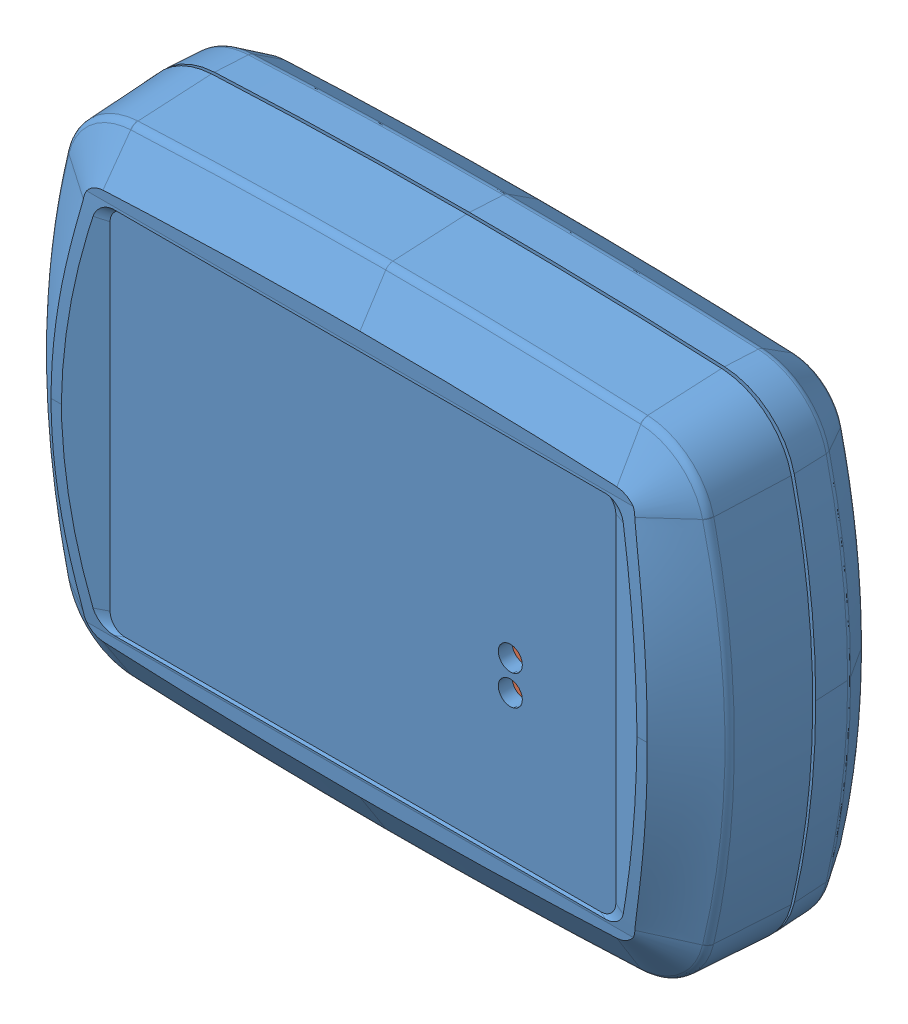
SolidWorks assembly СБ Peggy Receiver, configuration Default. Lengths in mm. (continued)
Components (placement in the parent): (continued)
- Печатная плата Peggy Receiver-1: Печатная плата Peggy Receiver [Default] at (11919.9713 53.7301 2.2215) x (0.000006 1 0) z (0 0 1) size (75.31 78.06 11.44) (continued)
  - Печатная плата Peggy Receiver(2)^Печатная плата Peggy Receiver-2: Печатная плата Peggy Receiver(2)^Печатная плата Peggy Receiver [Default] at origin size (75.31 78.06 11.44) (virtual) (continued)
    - DD1^Печатная плата Peggy Receiver(2)_Печатная плата Peggy Receiver-2: DD1^Печатная плата Peggy Receiver(2)_Печатная плата Peggy Receiver [Default] at origin size (16 15.9 2.23) (virtual) (continued)
      - User Library-RFM96W^DD1_Печатная плата Peggy Receiver(2)_Печатная плата Peggy Receiver-1: User Library-RFM96W^DD1_Печатная плата Peggy Receiver(2)_Печатная плата Peggy Receiver [Default] at (17.298 57.975 1.15) x (1 0 0) z (0 0 1) size (16 15.9 2.23) (virtual) (continued)
        - Designator9^User Library-RFM96W_DD1_Печатная плата Peggy Receiver(2)_Печатная плата Peggy Receiver-1: Designator9^User Library-RFM96W_DD1_Печатная плата Peggy Receiver(2)_Печатная плата Peggy Receiver [Default] at origin size (0.5 1 0.5) (virtual)
          - Cap0402^Designator9_User Library-RFM96W_DD1_Печатная плата Peggy Receiver(2)_Печатная плата Peggy Receiver-1: Cap0402^Designator9_User Library-RFM96W_DD1_Печатная плата Peggy Receiver(2)_Печатная плата Peggy Receiver [Default] at (2.8 5.98 0) x (0 -1 0) z (-1 0 0) size (1 0.5 0.5) (virtual)
        - Designator10^User Library-RFM96W_DD1_Печатная плата Peggy Receiver(2)_Печатная плата Peggy Receiver-1: Designator10^User Library-RFM96W_DD1_Печатная плата Peggy Receiver(2)_Печатная плата Peggy Receiver [Default] at origin size (0.5 1 0.5) (virtual)
          - Cap0402^Designator10_User Library-RFM96W_DD1_Печатная плата Peggy Receiver(2)_Печатная плата Peggy Receiver-1: Cap0402^Designator10_User Library-RFM96W_DD1_Печатная плата Peggy Receiver(2)_Печатная плата Peggy Receiver [Default] at (4.953 6.858 0) x (0 -1 0) z (-1 0 0) size (1 0.5 0.5) (virtual)
        - Designator11^User Library-RFM96W_DD1_Печатная плата Peggy Receiver(2)_Печатная плата Peggy Receiver-1: Designator11^User Library-RFM96W_DD1_Печатная плата Peggy Receiver(2)_Печатная плата Peggy Receiver [Default] at origin size (0.5 1 0.5) (virtual)
          - Cap0402^Designator11_User Library-RFM96W_DD1_Печатная плата Peggy Receiver(2)_Печатная плата Peggy Receiver-1: Cap0402^Designator11_User Library-RFM96W_DD1_Печатная плата Peggy Receiver(2)_Печатная плата Peggy Receiver [Default] at (6.35 11.557 0) x (0 1 0) z (1 0 0) size (1 0.5 0.5) (virtual)
        - Designator12^User Library-RFM96W_DD1_Печатная плата Peggy Receiver(2)_Печатная плата Peggy Receiver-1: Designator12^User Library-RFM96W_DD1_Печатная плата Peggy Receiver(2)_Печатная плата Peggy Receiver [Default] at origin size (1 0.5 0.5) (virtual)
          - Cap0402^Designator12_User Library-RFM96W_DD1_Печатная плата Peggy Receiver(2)_Печатная плата Peggy Receiver-1: Cap0402^Designator12_User Library-RFM96W_DD1_Печатная плата Peggy Receiver(2)_Печатная плата Peggy Receiver [Default] at (5.461 8.128 0) x (1 0 0) z (0 -1 0) size (1 0.5 0.5) (virtual)
        - Designator13^User Library-RFM96W_DD1_Печатная плата Peggy Receiver(2)_Печатная плата Peggy Receiver-1: Designator13^User Library-RFM96W_DD1_Печатная плата Peggy Receiver(2)_Печатная плата Peggy Receiver [Default] at origin size (0.5 1 0.5) (virtual)
          - Cap0402^Designator13_User Library-RFM96W_DD1_Печатная плата Peggy Receiver(2)_Печатная плата Peggy Receiver-1: Cap0402^Designator13_User Library-RFM96W_DD1_Печатная плата Peggy Receiver(2)_Печатная плата Peggy Receiver [Default] at (3.937 6.858 0) x (0 1 0) z (1 0 0) size (1 0.5 0.5) (virtual)
        - Designator15^User Library-RFM96W_DD1_Печатная плата Peggy Receiver(2)_Печатная плата Peggy Receiver-1: Designator15^User Library-RFM96W_DD1_Печатная плата Peggy Receiver(2)_Печатная плата Peggy Receiver [Default] at origin size (0.52 1.02 0.37) (virtual)
          - SW3dPS-inductor_0402_white^Designator15_User Library-RFM96W_DD1_Печатная плата Peggy Receiver(2)_Печатная плата Peggy Receiver-1: SW3dPS-inductor_0402_white^Designator15_User Library-RFM96W_DD1_Печатная плата Peggy Receiver(2)_Печатная плата Peggy Receiver [Default] at (13.208 12.446 0) x (1 0 0) z (0 -1 0) size (0.52 0.37 1.02) (virtual)
        - Designator17^User Library-RFM96W_DD1_Печатная плата Peggy Receiver(2)_Печатная плата Peggy Receiver-1: Designator17^User Library-RFM96W_DD1_Печатная плата Peggy Receiver(2)_Печатная плата Peggy Receiver [Default] at origin size (1.02 0.52 0.37) (virtual)
          - SW3dPS-inductor_0402_white^Designator17_User Library-RFM96W_DD1_Печатная плата Peggy Receiver(2)_Печатная плата Peggy Receiver-1: SW3dPS-inductor_0402_white^Designator17_User Library-RFM96W_DD1_Печатная плата Peggy Receiver(2)_Печатная плата Peggy Receiver [Default] at (8.636 8.89 0) x (0 1 0) z (1 0 0) size (0.52 0.37 1.02) (virtual)
        - Designator18^User Library-RFM96W_DD1_Печатная плата Peggy Receiver(2)_Печатная плата Peggy Receiver-1: Designator18^User Library-RFM96W_DD1_Печатная плата Peggy Receiver(2)_Печатная плата Peggy Receiver [Default] at origin size (1.02 0.52 0.37) (virtual)
          - SW3dPS-inductor_0402_white^Designator18_User Library-RFM96W_DD1_Печатная плата Peggy Receiver(2)_Печатная плата Peggy Receiver-1: SW3dPS-inductor_0402_white^Designator18_User Library-RFM96W_DD1_Печатная плата Peggy Receiver(2)_Печатная плата Peggy Receiver [Default] at (9.398 10.414 0) x (0 1 0) z (1 0 0) size (0.52 0.37 1.02) (virtual)
        - Designator19^User Library-RFM96W_DD1_Печатная плата Peggy Receiver(2)_Печатная плата Peggy Receiver-1: Designator19^User Library-RFM96W_DD1_Печатная плата Peggy Receiver(2)_Печатная плата Peggy Receiver [Default] at origin size (1.02 0.52 0.37) (virtual)
          - SW3dPS-inductor_0402_white^Designator19_User Library-RFM96W_DD1_Печатная плата Peggy Receiver(2)_Печатная плата Peggy Receiver-1: SW3dPS-inductor_0402_white^Designator19_User Library-RFM96W_DD1_Печатная плата Peggy Receiver(2)_Печатная плата Peggy Receiver [Default] at (8.636 12.319 0) x (0 1 0) z (1 0 0) size (0.52 0.37 1.02) (virtual)
        - Designator20^User Library-RFM96W_DD1_Печатная плата Peggy Receiver(2)_Печатная плата Peggy Receiver-1: Designator20^User Library-RFM96W_DD1_Печатная плата Peggy Receiver(2)_Печатная плата Peggy Receiver [Default] at origin size (1.02 0.52 0.37) (virtual)
          - SW3dPS-inductor_0402_white^Designator20_User Library-RFM96W_DD1_Печатная плата Peggy Receiver(2)_Печатная плата Peggy Receiver-1: SW3dPS-inductor_0402_white^Designator20_User Library-RFM96W_DD1_Печатная плата Peggy Receiver(2)_Печатная плата Peggy Receiver [Default] at (10.668 12.319 0) x (0 1 0) z (1 0 0) size (0.52 0.37 1.02) (virtual)
        - Designator21^User Library-RFM96W_DD1_Печатная плата Peggy Receiver(2)_Печатная плата Peggy Receiver-1: Designator21^User Library-RFM96W_DD1_Печатная плата Peggy Receiver(2)_Печатная плата Peggy Receiver [Default] at origin size (1 0.5 0.5) (virtual)
          - Cap0402^Designator21_User Library-RFM96W_DD1_Печатная плата Peggy Receiver(2)_Печатная плата Peggy Receiver-1: Cap0402^Designator21_User Library-RFM96W_DD1_Печатная плата Peggy Receiver(2)_Печатная плата Peggy Receiver [Default] at (10.668 10.414 0) x (-1 0 0) z (0 1 0) size (1 0.5 0.5) (virtual)
        - Designator22^User Library-RFM96W_DD1_Печатная плата Peggy Receiver(2)_Печатная плата Peggy Receiver-1: Designator22^User Library-RFM96W_DD1_Печатная плата Peggy Receiver(2)_Печатная плата Peggy Receiver [Default] at origin size (0.5 1 0.5) (virtual)
          - Cap0402^Designator22_User Library-RFM96W_DD1_Печатная плата Peggy Receiver(2)_Печатная плата Peggy Receiver-1: Cap0402^Designator22_User Library-RFM96W_DD1_Печатная плата Peggy Receiver(2)_Печатная плата Peggy Receiver [Default] at (8.255 10.922 0) x (0 1 0) z (1 0 0) size (1 0.5 0.5) (virtual)
        - Designator23^User Library-RFM96W_DD1_Печатная плата Peggy Receiver(2)_Печатная плата Peggy Receiver-1: Designator23^User Library-RFM96W_DD1_Печатная плата Peggy Receiver(2)_Печатная плата Peggy Receiver [Default] at origin size (1 0.5 0.5) (virtual)
          - Cap0402^Designator23_User Library-RFM96W_DD1_Печатная плата Peggy Receiver(2)_Печатная плата Peggy Receiver-1: Cap0402^Designator23_User Library-RFM96W_DD1_Печатная плата Peggy Receiver(2)_Печатная плата Peggy Receiver [Default] at (6.858 14.859 0) x (-1 0 0) z (0 1 0) size (1 0.5 0.5) (virtual)
        - Designator24^User Library-RFM96W_DD1_Печатная плата Peggy Receiver(2)_Печатная плата Peggy Receiver-1: Designator24^User Library-RFM96W_DD1_Печатная плата Peggy Receiver(2)_Печатная плата Peggy Receiver [Default] at origin size (1 0.5 0.5) (virtual)
          - Cap0402^Designator24_User Library-RFM96W_DD1_Печатная плата Peggy Receiver(2)_Печатная плата Peggy Receiver-1: Cap0402^Designator24_User Library-RFM96W_DD1_Печатная плата Peggy Receiver(2)_Печатная плата Peggy Receiver [Default] at (12.827 13.843 0) x (-1 0 0) z (0 1 0) size (1 0.5 0.5) (virtual)
        - Designator25^User Library-RFM96W_DD1_Печатная плата Peggy Receiver(2)_Печатная плата Peggy Receiver-1: Designator25^User Library-RFM96W_DD1_Печатная плата Peggy Receiver(2)_Печатная плата Peggy Receiver [Default] at origin size (0.5 1 0.5) (virtual)
          - Cap0402^Designator25_User Library-RFM96W_DD1_Печатная плата Peggy Receiver(2)_Печатная плата Peggy Receiver-1: Cap0402^Designator25_User Library-RFM96W_DD1_Печатная плата Peggy Receiver(2)_Печатная плата Peggy Receiver [Default] at (7.366 11.938 0) x (0 -1 0) z (-1 0 0) size (1 0.5 0.5) (virtual)
        - Designator26^User Library-RFM96W_DD1_Печатная плата Peggy Receiver(2)_Печатная плата Peggy Receiver-1: Designator26^User Library-RFM96W_DD1_Печатная плата Peggy Receiver(2)_Печатная плата Peggy Receiver [Default] at origin size (0.5 1 0.5) (virtual)
          - Cap0402^Designator26_User Library-RFM96W_DD1_Печатная плата Peggy Receiver(2)_Печатная плата Peggy Receiver-1: Cap0402^Designator26_User Library-RFM96W_DD1_Печатная плата Peggy Receiver(2)_Печатная плата Peggy Receiver [Default] at (12.319 12.446 0) x (0 -1 0) z (-1 0 0) size (1 0.5 0.5) (virtual)
        - Designator27^User Library-RFM96W_DD1_Печатная плата Peggy Receiver(2)_Печатная плата Peggy Receiver-1: Designator27^User Library-RFM96W_DD1_Печатная плата Peggy Receiver(2)_Печатная плата Peggy Receiver [Default] at origin size (1 0.5 0.5) (virtual)
          - Cap0402^Designator27_User Library-RFM96W_DD1_Печатная плата Peggy Receiver(2)_Печатная плата Peggy Receiver-1: Cap0402^Designator27_User Library-RFM96W_DD1_Печатная плата Peggy Receiver(2)_Печатная плата Peggy Receiver [Default] at (12.827 14.986 0) x (-1 0 0) z (0 1 0) size (1 0.5 0.5) (virtual)
        - Designator28^User Library-RFM96W_DD1_Печатная плата Peggy Receiver(2)_Печатная плата Peggy Receiver-1: Designator28^User Library-RFM96W_DD1_Печатная плата Peggy Receiver(2)_Печатная плата Peggy Receiver [Default] at origin size (0.5 1 0.5) (virtual)
          - Cap0402^Designator28_User Library-RFM96W_DD1_Печатная плата Peggy Receiver(2)_Печатная плата Peggy Receiver-1: Cap0402^Designator28_User Library-RFM96W_DD1_Печатная плата Peggy Receiver(2)_Печатная плата Peggy Receiver [Default] at (9.652 11.684 0) x (0 -1 0) z (-1 0 0) size (1 0.5 0.5) (virtual)
        - Designator29^User Library-RFM96W_DD1_Печатная плата Peggy Receiver(2)_Печатная плата Peggy Receiver-1: Designator29^User Library-RFM96W_DD1_Печатная плата Peggy Receiver(2)_Печатная плата Peggy Receiver [Default] at origin size (0.5 1 0.5) (virtual)
          - Cap0402^Designator29_User Library-RFM96W_DD1_Печатная плата Peggy Receiver(2)_Печатная плата Peggy Receiver-1: Cap0402^Designator29_User Library-RFM96W_DD1_Печатная плата Peggy Receiver(2)_Печатная плата Peggy Receiver [Default] at (13.208 9.779 0) x (0 -1 0) z (-1 0 0) size (1 0.5 0.5) (virtual)
        - Designator27_2^User Library-RFM96W_DD1_Печатная плата Peggy Receiver(2)_Печатная плата Peggy Receiver-1: Designator27_2^User Library-RFM96W_DD1_Печатная плата Peggy Receiver(2)_Печатная плата Peggy Receiver [Default] at origin size (2.43 2.79 1.09) (virtual)
          - SW3dPS-SOT-23-6^Designator27_2_User Library-RFM96W_DD1_Печатная плата Peggy Receiver(2)_Печатная плата Peggy Receiver-1: SW3dPS-SOT-23-6^Designator27_2_User Library-RFM96W_DD1_Печатная плата Peggy Receiver(2)_Печатная плата Peggy Receiver [Default] at (9.0742 15.0495 0) x (0 -1 0) z (0 0 1) size (2.79 2.43 1.09) (virtual)
        - Designator2^User Library-RFM96W_DD1_Печатная плата Peggy Receiver(2)_Печатная плата Peggy Receiver-1: Designator2^User Library-RFM96W_DD1_Печатная плата Peggy Receiver(2)_Печатная плата Peggy Receiver [Default] at origin size (5.04 5.04 0.9) (virtual)
          - QFN28^Designator2_User Library-RFM96W_DD1_Печатная плата Peggy Receiver(2)_Печатная плата Peggy Receiver-1: QFN28^Designator2_User Library-RFM96W_DD1_Печатная плата Peggy Receiver(2)_Печатная плата Peggy Receiver [Default] at (9.97 5.42 0) x (0 -1 0) z (-1 0 0) size (5.04 0.9 5.04) (virtual)
        - Designator5^User Library-RFM96W_DD1_Печатная плата Peggy Receiver(2)_Печатная плата Peggy Receiver-1: Designator5^User Library-RFM96W_DD1_Печатная плата Peggy Receiver(2)_Печатная плата Peggy Receiver [Default] at origin size (0.5 1 0.5) (virtual)
          - Cap0402^Designator5_User Library-RFM96W_DD1_Печатная плата Peggy Receiver(2)_Печатная плата Peggy Receiver-1: Cap0402^Designator5_User Library-RFM96W_DD1_Печатная плата Peggy Receiver(2)_Печатная плата Peggy Receiver [Default] at (12.192 1.27 0) x (0 -1 0) z (-1 0 0) size (1 0.5 0.5) (virtual)
        - Designator1^User Library-RFM96W_DD1_Печатная плата Peggy Receiver(2)_Печатная плата Peggy Receiver-1: Designator1^User Library-RFM96W_DD1_Печатная плата Peggy Receiver(2)_Печатная плата Peggy Receiver [Default] at origin size (2.5 3.2 0.7) (virtual)
          - TXC_7M^Designator1_User Library-RFM96W_DD1_Печатная плата Peggy Receiver(2)_Печатная плата Peggy Receiver-1: TXC_7M^Designator1_User Library-RFM96W_DD1_Печатная плата Peggy Receiver(2)_Печатная плата Peggy Receiver [Default] at (4.1911 2.286 0) x (0 1 0) z (1 0 0) size (3.2 0.7 2.5) (virtual)
        - Open CASCADE STEP translator 6.5 1.29^User Library-RFM96W_DD1_Печатная плата Peggy Receiver(2)_Печатная плата Peggy Receiver-1: Open CASCADE STEP translator 6.5 1.29^User Library-RFM96W_DD1_Печатная плата Peggy Receiver(2)_Печатная плата Peggy Receiver [Default] at origin size (0.5 1 0.35) (virtual)
          - Res0402^Open CASCADE STEP translator 6.5 1.29_User Library-RFM96W_DD1_Печатная плата Peggy Receiver(2)_Печатная плата Peggy Receiver-1: Res0402^Open CASCADE STEP translator 6.5 1.29_User Library-RFM96W_DD1_Печатная плата Peggy Receiver(2)_Печатная плата Peggy Receiver [Default] at (2.794 7.62 0) x (0 1 0) z (1 0 0) size (1 0.35 0.5) (virtual)
        - 1^User Library-RFM96W_DD1_Печатная плата Peggy Receiver(2)_Печатная плата Peggy Receiver-1: 1^User Library-RFM96W_DD1_Печатная плата Peggy Receiver(2)_Печатная плата Peggy Receiver [Default] at origin size (0.5 1 0.35) (virtual)
          - Res0402^1_User Library-RFM96W_DD1_Печатная плата Peggy Receiver(2)_Печатная плата Peggy Receiver-1: Res0402^1_User Library-RFM96W_DD1_Печатная плата Peggy Receiver(2)_Печатная плата Peggy Receiver [Default] at (2.921 9.652 0) x (0 1 0) z (1 0 0) size (1 0.35 0.5) (virtual)
        - 2^User Library-RFM96W_DD1_Печатная плата Peggy Receiver(2)_Печатная плата Peggy Receiver-1: 2^User Library-RFM96W_DD1_Печатная плата Peggy Receiver(2)_Печатная плата Peggy Receiver [Default] at origin size (0.5 1 0.35) (virtual)
          - Res0402^2_User Library-RFM96W_DD1_Печатная плата Peggy Receiver(2)_Печатная плата Peggy Receiver-1: Res0402^2_User Library-RFM96W_DD1_Печатная плата Peggy Receiver(2)_Печатная плата Peggy Receiver [Default] at (4.064 9.652 0) x (0 1 0) z (1 0 0) size (1 0.35 0.5) (virtual)
        - Open CASCADE STEP translator 6.5 1.32^User Library-RFM96W_DD1_Печатная плата Peggy Receiver(2)_Печатная плата Peggy Receiver-1: Open CASCADE STEP translator 6.5 1.32^User Library-RFM96W_DD1_Печатная плата Peggy Receiver(2)_Печатная плата Peggy Receiver [Default] at origin size (3.03 2.48 1.12) (virtual)
          - User_Library-3-lead_sot23-3^Open CASCADE STEP translator 6.5 1.32_User Library-RFM96W_DD1_Печатная плата Peggy Receiver(2)_Печатная плата Peggy Receiver-1: User_Library-3-lead_sot23-3^Open CASCADE STEP translator 6.5 1.32_User Library-RFM96W_DD1_Печатная плата Peggy Receiver(2)_Печатная плата Peggy Receiver [Default] at (3.9981 12.3031 0.35) x (1 0 0) z (0 -1 0) size (3.03 1.12 2.48) (virtual)
        - 3^User Library-RFM96W_DD1_Печатная плата Peggy Receiver(2)_Печатная плата Peggy Receiver-1: 3^User Library-RFM96W_DD1_Печатная плата Peggy Receiver(2)_Печатная плата Peggy Receiver [Default] at origin size (1 0.5 0.35) (virtual)
          - Res0402^3_User Library-RFM96W_DD1_Печатная плата Peggy Receiver(2)_Печатная плата Peggy Receiver-1: Res0402^3_User Library-RFM96W_DD1_Печатная плата Peggy Receiver(2)_Печатная плата Peggy Receiver [Default] at (4.445 14.859 0) x (-1 0 0) z (0 1 0) size (1 0.35 0.5) (virtual)
        - Designator31^User Library-RFM96W_DD1_Печатная плата Peggy Receiver(2)_Печатная плата Peggy Receiver-1: Designator31^User Library-RFM96W_DD1_Печатная плата Peggy Receiver(2)_Печатная плата Peggy Receiver [Default] at origin size (1 0.5 0.5) (virtual)
          - Cap0402^Designator31_User Library-RFM96W_DD1_Печатная плата Peggy Receiver(2)_Печатная плата Peggy Receiver-1: Cap0402^Designator31_User Library-RFM96W_DD1_Печатная плата Peggy Receiver(2)_Печатная плата Peggy Receiver [Default] at (8.636 9.652 0) x (-1 0 0) z (0 1 0) size (1 0.5 0.5) (virtual)
        - Designator32^User Library-RFM96W_DD1_Печатная плата Peggy Receiver(2)_Печатная плата Peggy Receiver-1: Designator32^User Library-RFM96W_DD1_Печатная плата Peggy Receiver(2)_Печатная плата Peggy Receiver [Default] at origin size (1 0.5 0.5) (virtual)
          - Cap0402^Designator32_User Library-RFM96W_DD1_Печатная плата Peggy Receiver(2)_Печатная плата Peggy Receiver-1: Cap0402^Designator32_User Library-RFM96W_DD1_Печатная плата Peggy Receiver(2)_Печатная плата Peggy Receiver [Default] at (10.668 9.652 0) x (-1 0 0) z (0 1 0) size (1 0.5 0.5) (virtual)
        - Free-Models^User Library-RFM96W_DD1_Печатная плата Peggy Receiver(2)_Печатная плата Peggy Receiver-1: Free-Models^User Library-RFM96W_DD1_Печатная плата Peggy Receiver(2)_Печатная плата Peggy Receiver [Default] at origin size (16 15.3 1.16) (virtual)
          - Goldcontact^Free-Models_User Library-RFM96W_DD1_Печатная плата Peggy Receiver(2)_Печатная плата Peggy Receiver-1: Goldcontact^Free-Models_User Library-RFM96W_DD1_Печатная плата Peggy Receiver(2)_Печатная плата Peggy Receiver [Default] at (0.56 1 -1.14) x (-1 0 0) z (0 1 0) size (1.77 1.16 1.3) (virtual)
          - Goldcontact^Free-Models_User Library-RFM96W_DD1_Печатная плата Peggy Receiver(2)_Печатная плата Peggy Receiver-2: Goldcontact^Free-Models_User Library-RFM96W_DD1_Печатная плата Peggy Receiver(2)_Печатная плата Peggy Receiver [Default] at (0.56 3 -1.14) x (-1 0 0) z (0 1 0) size (1.77 1.16 1.3) (virtual)
          - Goldcontact^Free-Models_User Library-RFM96W_DD1_Печатная плата Peggy Receiver(2)_Печатная плата Peggy Receiver-3: Goldcontact^Free-Models_User Library-RFM96W_DD1_Печатная плата Peggy Receiver(2)_Печатная плата Peggy Receiver [Default] at (0.56 5 -1.14) x (-1 0 0) z (0 1 0) size (1.77 1.16 1.3) (virtual)
          - Goldcontact^Free-Models_User Library-RFM96W_DD1_Печатная плата Peggy Receiver(2)_Печатная плата Peggy Receiver-4: Goldcontact^Free-Models_User Library-RFM96W_DD1_Печатная плата Peggy Receiver(2)_Печатная плата Peggy Receiver [Default] at (0.56 7 -1.14) x (-1 0 0) z (0 1 0) size (1.77 1.16 1.3) (virtual)
          - Goldcontact^Free-Models_User Library-RFM96W_DD1_Печатная плата Peggy Receiver(2)_Печатная плата Peggy Receiver-5: Goldcontact^Free-Models_User Library-RFM96W_DD1_Печатная плата Peggy Receiver(2)_Печатная плата Peggy Receiver [Default] at (0.56 9 -1.14) x (-1 0 0) z (0 1 0) size (1.77 1.16 1.3) (virtual)
          - Goldcontact^Free-Models_User Library-RFM96W_DD1_Печатная плата Peggy Receiver(2)_Печатная плата Peggy Receiver-6: Goldcontact^Free-Models_User Library-RFM96W_DD1_Печатная плата Peggy Receiver(2)_Печатная плата Peggy Receiver [Default] at (0.56 11 -1.14) x (-1 0 0) z (0 1 0) size (1.77 1.16 1.3) (virtual)
          - Goldcontact^Free-Models_User Library-RFM96W_DD1_Печатная плата Peggy Receiver(2)_Печатная плата Peggy Receiver-7: Goldcontact^Free-Models_User Library-RFM96W_DD1_Печатная плата Peggy Receiver(2)_Печатная плата Peggy Receiver [Default] at (0.56 13 -1.14) x (-1 0 0) z (0 1 0) size (1.77 1.16 1.3) (virtual)
          - Goldcontact^Free-Models_User Library-RFM96W_DD1_Печатная плата Peggy Receiver(2)_Печатная плата Peggy Receiver-8: Goldcontact^Free-Models_User Library-RFM96W_DD1_Печатная плата Peggy Receiver(2)_Печатная плата Peggy Receiver [Default] at (0.56 15 -1.14) x (-1 0 0) z (0 1 0) size (1.77 1.16 1.3) (virtual)
          - Goldcontact^Free-Models_User Library-RFM96W_DD1_Печатная плата Peggy Receiver(2)_Печатная плата Peggy Receiver-9: Goldcontact^Free-Models_User Library-RFM96W_DD1_Печатная плата Peggy Receiver(2)_Печатная плата Peggy Receiver [Default] at (15.442 15 -1.14) x (1 0 0) z (0 -1 0) size (1.77 1.16 1.3) (virtual)
          - Goldcontact^Free-Models_User Library-RFM96W_DD1_Печатная плата Peggy Receiver(2)_Печатная плата Peggy Receiver-10: Goldcontact^Free-Models_User Library-RFM96W_DD1_Печатная плата Peggy Receiver(2)_Печатная плата Peggy Receiver [Default] at (15.442 13 -1.14) x (1 0 0) z (0 -1 0) size (1.77 1.16 1.3) (virtual)
          - Goldcontact^Free-Models_User Library-RFM96W_DD1_Печатная плата Peggy Receiver(2)_Печатная плата Peggy Receiver-11: Goldcontact^Free-Models_User Library-RFM96W_DD1_Печатная плата Peggy Receiver(2)_Печатная плата Peggy Receiver [Default] at (15.442 11 -1.14) x (1 0 0) z (0 -1 0) size (1.77 1.16 1.3) (virtual)
          - Goldcontact^Free-Models_User Library-RFM96W_DD1_Печатная плата Peggy Receiver(2)_Печатная плата Peggy Receiver-12: Goldcontact^Free-Models_User Library-RFM96W_DD1_Печатная плата Peggy Receiver(2)_Печатная плата Peggy Receiver [Default] at (15.442 9 -1.14) x (1 0 0) z (0 -1 0) size (1.77 1.16 1.3) (virtual)
          - Goldcontact^Free-Models_User Library-RFM96W_DD1_Печатная плата Peggy Receiver(2)_Печатная плата Peggy Receiver-13: Goldcontact^Free-Models_User Library-RFM96W_DD1_Печатная плата Peggy Receiver(2)_Печатная плата Peggy Receiver [Default] at (15.442 7 -1.14) x (1 0 0) z (0 -1 0) size (1.77 1.16 1.3) (virtual)
          - Goldcontact^Free-Models_User Library-RFM96W_DD1_Печатная плата Peggy Receiver(2)_Печатная плата Peggy Receiver-14: Goldcontact^Free-Models_User Library-RFM96W_DD1_Печатная плата Peggy Receiver(2)_Печатная плата Peggy Receiver [Default] at (15.442 5 -1.14) x (1 0 0) z (0 -1 0) size (1.77 1.16 1.3) (virtual)
          - Goldcontact^Free-Models_User Library-RFM96W_DD1_Печатная плата Peggy Receiver(2)_Печатная плата Peggy Receiver-15: Goldcontact^Free-Models_User Library-RFM96W_DD1_Печатная плата Peggy Receiver(2)_Печатная плата Peggy Receiver [Default] at (15.442 3 -1.14) x (1 0 0) z (0 -1 0) size (1.77 1.16 1.3) (virtual)
          - Goldcontact^Free-Models_User Library-RFM96W_DD1_Печатная плата Peggy Receiver(2)_Печатная плата Peggy Receiver-16: Goldcontact^Free-Models_User Library-RFM96W_DD1_Печатная плата Peggy Receiver(2)_Печатная плата Peggy Receiver [Default] at (15.442 1 -1.14) x (1 0 0) z (0 -1 0) size (1.77 1.16 1.3) (virtual)
        - Board-4^User Library-RFM96W_DD1_Печатная плата Peggy Receiver(2)_Печатная плата Peggy Receiver-1: Board-4^User Library-RFM96W_DD1_Печатная плата Peggy Receiver(2)_Печатная плата Peggy Receiver [Default] at (0 0 -1.1204) size (15.9 15.9 1.12) (virtual)
    - D2^Печатная плата Peggy Receiver(2)_Печатная плата Peggy Receiver-2: D2^Печатная плата Peggy Receiver(2)_Печатная плата Peggy Receiver [Default] at origin size (3 3 1.3) (virtual)
      - SOT23-5-1^D2_Печатная плата Peggy Receiver(2)_Печатная плата Peggy Receiver-1: SOT23-5-1^D2_Печатная плата Peggy Receiver(2)_Печатная плата Peggy Receiver [Default] at (9.1731 22.6912 0) x (-1 0 0) z (0 0 1) size (3 3 1.3) (virtual)
    - C14^Печатная плата Peggy Receiver(2)_Печатная плата Peggy Receiver-2: C14^Печатная плата Peggy Receiver(2)_Печатная плата Peggy Receiver [Default] at origin size (1.6 0.8 0.3) (virtual)
      - SW3dPS-0603 SMD Capacitor^C14_Печатная плата Peggy Receiver(2)_Печатная плата Peggy Receiver-1: SW3dPS-0603 SMD Capacitor^C14_Печатная плата Peggy Receiver(2)_Печатная плата Peggy Receiver [Default] at (18.8091 16.273 0) x (1 0 0) z (0 -1 0) size (1.6 0.3 0.8) (virtual)
    - C10^Печатная плата Peggy Receiver(2)_Печатная плата Peggy Receiver-2: C10^Печатная плата Peggy Receiver(2)_Печатная плата Peggy Receiver [Default] at origin size (0.8 1.6 0.3) (virtual)
      - SW3dPS-0603 SMD Capacitor^C10_Печатная плата Peggy Receiver(2)_Печатная плата Peggy Receiver-1: SW3dPS-0603 SMD Capacitor^C10_Печатная плата Peggy Receiver(2)_Печатная плата Peggy Receiver [Default] at (45.2091 39.5728 0) x (0 -1 0) z (-1 0 0) size (1.6 0.3 0.8) (virtual)
    - C9^Печатная плата Peggy Receiver(2)_Печатная плата Peggy Receiver-2: C9^Печатная плата Peggy Receiver(2)_Печатная плата Peggy Receiver [Default] at origin size (0.8 1.6 0.3) (virtual)
      - SW3dPS-0603 SMD Capacitor^C9_Печатная плата Peggy Receiver(2)_Печатная плата Peggy Receiver-1: SW3dPS-0603 SMD Capacitor^C9_Печатная плата Peggy Receiver(2)_Печатная плата Peggy Receiver [Default] at (45.3089 31.473 0) x (0 1 0) z (1 0 0) size (1.6 0.3 0.8) (virtual)
    - C8^Печатная плата Peggy Receiver(2)_Печатная плата Peggy Receiver-2: C8^Печатная плата Peggy Receiver(2)_Печатная плата Peggy Receiver [Default] at origin size (1.6 0.8 0.3) (virtual)
      - SW3dPS-0603 SMD Capacitor^C8_Печатная плата Peggy Receiver(2)_Печатная плата Peggy Receiver-1: SW3dPS-0603 SMD Capacitor^C8_Печатная плата Peggy Receiver(2)_Печатная плата Peggy Receiver [Default] at (33.6089 27.7728 0) x (-1 0 0) z (0 1 0) size (1.6 0.3 0.8) (virtual)
    - C7^Печатная плата Peggy Receiver(2)_Печатная плата Peggy Receiver-2: C7^Печатная плата Peggy Receiver(2)_Печатная плата Peggy Receiver [Default] at origin size (0.8 1.6 0.3) (virtual)
      - SW3dPS-0603 SMD Capacitor^C7_Печатная плата Peggy Receiver(2)_Печатная плата Peggy Receiver-1: SW3dPS-0603 SMD Capacitor^C7_Печатная плата Peggy Receiver(2)_Печатная плата Peggy Receiver [Default] at (28.9091 40.9728 0) x (0 -1 0) z (-1 0 0) size (1.6 0.3 0.8) (virtual)
    - C3^Печатная плата Peggy Receiver(2)_Печатная плата Peggy Receiver-2: C3^Печатная плата Peggy Receiver(2)_Печатная плата Peggy Receiver [Default] at origin size (1.75 0.95 0.87) (virtual)
      - 6665910208^C3_Печатная плата Peggy Receiver(2)_Печатная плата Peggy Receiver-1: 6665910208^C3_Печатная плата Peggy Receiver(2)_Печатная плата Peggy Receiver [Default] at (26.5 40.2 0) x (-1 0 0) z (0 0 1) size (1.75 0.95 0.87) (virtual)
        - Terminal-2^6665910208_C3_Печатная плата Peggy Receiver(2)_Печатная плата Peggy Receiver-1: Terminal-2^6665910208_C3_Печатная плата Peggy Receiver(2)_Печатная плата Peggy Receiver [Default] at (-0.875 -0.475 0) size (1.75 0.95 0.87) (virtual)
          - Open CASCADE STEP translator 6.8 127.1.1^Terminal-2_6665910208_C3_Печатная плата Peggy Receiver(2)_Печатная плата Peggy Receiver-1: Open CASCADE STEP translator 6.8 127.1.1^Terminal-2_6665910208_C3_Печатная плата Peggy Receiver(2)_Печатная плата Peggy Receiver [Default] at origin size (0.2 0.95 0.87) (virtual)
          - Open CASCADE STEP translator 6.8 127.1.2^Terminal-2_6665910208_C3_Печатная плата Peggy Receiver(2)_Печатная плата Peggy Receiver-1: Open CASCADE STEP translator 6.8 127.1.2^Terminal-2_6665910208_C3_Печатная плата Peggy Receiver(2)_Печатная плата Peggy Receiver [Default] at origin size (0.2 0.95 0.87) (virtual)
        - Mid_Body-5^6665910208_C3_Печатная плата Peggy Receiver(2)_Печатная плата Peggy Receiver-1: Mid_Body-5^6665910208_C3_Печатная плата Peggy Receiver(2)_Печатная плата Peggy Receiver [Default] at (-0.875 -0.475 0) size (1.35 0.95 0.87) (virtual)
          - Open CASCADE STEP translator 6.8 127.2.1^Mid_Body-5_6665910208_C3_Печатная плата Peggy Receiver(2)_Печатная плата Peggy Receiver-1: Open CASCADE STEP translator 6.8 127.2.1^Mid_Body-5_6665910208_C3_Печатная плата Peggy Receiver(2)_Печатная плата Peggy Receiver [Default] at origin size (1.35 0.95 0.87) (virtual)
    - C2^Печатная плата Peggy Receiver(2)_Печатная плата Peggy Receiver-2: C2^Печатная плата Peggy Receiver(2)_Печатная плата Peggy Receiver [Default] at origin size (1.75 0.95 0.87) (virtual)
      - 6665910368^C2_Печатная плата Peggy Receiver(2)_Печатная плата Peggy Receiver-1: 6665910368^C2_Печатная плата Peggy Receiver(2)_Печатная плата Peggy Receiver [Default] at (28.109 31.9729 0) x (1 0 0) z (0 0 1) size (1.75 0.95 0.87) (virtual)
        - Terminal-3^6665910368_C2_Печатная плата Peggy Receiver(2)_Печатная плата Peggy Receiver-1: Terminal-3^6665910368_C2_Печатная плата Peggy Receiver(2)_Печатная плата Peggy Receiver [Default] at (-0.875 -0.475 0) size (1.75 0.95 0.87) (virtual)
          - Open CASCADE STEP translator 6.8 127.1.1-6^Terminal-3_6665910368_C2_Печатная плата Peggy Receiver(2)_Печатная плата Peggy Receiver-1: Open CASCADE STEP translator 6.8 127.1.1-6^Terminal-3_6665910368_C2_Печатная плата Peggy Receiver(2)_Печатная плата Peggy Receiver [Default] at origin size (0.2 0.95 0.87) (virtual)
          - Open CASCADE STEP translator 6.8 127.1.2-7^Terminal-3_6665910368_C2_Печатная плата Peggy Receiver(2)_Печатная плата Peggy Receiver-1: Open CASCADE STEP translator 6.8 127.1.2-7^Terminal-3_6665910368_C2_Печатная плата Peggy Receiver(2)_Печатная плата Peggy Receiver [Default] at origin size (0.2 0.95 0.87) (virtual)
        - Mid_Body-1-8^6665910368_C2_Печатная плата Peggy Receiver(2)_Печатная плата Peggy Receiver-1: Mid_Body-1-8^6665910368_C2_Печатная плата Peggy Receiver(2)_Печатная плата Peggy Receiver [Default] at (-0.875 -0.475 0) size (1.35 0.95 0.87) (virtual)
          - Open CASCADE STEP translator 6.8 127.2.1-9^Mid_Body-1-8_6665910368_C2_Печатная плата Peggy Receiver(2)_Печатная плата Peggy Receiver-1: Open CASCADE STEP translator 6.8 127.2.1-9^Mid_Body-1-8_6665910368_C2_Печатная плата Peggy Receiver(2)_Печатная плата Peggy Receiver [Default] at origin size (1.35 0.95 0.87) (virtual)
    - C1^Печатная плата Peggy Receiver(2)_Печатная плата Peggy Receiver-2: C1^Печатная плата Peggy Receiver(2)_Печатная плата Peggy Receiver [Default] at origin size (1.6 0.8 0.3) (virtual)
      - SW3dPS-0603 SMD Capacitor^C1_Печатная плата Peggy Receiver(2)_Печатная плата Peggy Receiver-1: SW3dPS-0603 SMD Capacitor^C1_Печатная плата Peggy Receiver(2)_Печатная плата Peggy Receiver [Default] at (29.6089 45.3728 0) x (-1 0 0) z (0 1 0) size (1.6 0.3 0.8) (virtual)
Mates (geometry in assembly coordinates):
- Concentric1: concentric aligned: cylinder of G1910-1 through (11916.7208 124.2891 1.81) axis (0 0 1) radius 1.125; circle of Печатная плата Peggy Receiver-1/Печатная плата Peggy Receiver(2)^Печатная плата Peggy Receiver-2/Board^Печатная плата Peggy Receiver(2)_Печатная плата Peggy Receiver-2/Open CASCADE STEP translator 7.5 1.1.1^Board_Печатная плата Peggy Receiver(2)_Печатная плата Peggy Receiver-1
- Concentric2: concentric anti-aligned: cylinder of G1910-1 through (11916.7214 60.7891 1.81) axis (0 0 -1) radius 1.125; circle of Печатная плата Peggy Receiver-1/Печатная плата Peggy Receiver(2)^Печатная плата Peggy Receiver-2/Board^Печатная плата Peggy Receiver(2)_Печатная плата Peggy Receiver-2/Open CASCADE STEP translator 7.5 1.1.1^Board_Печатная плата Peggy Receiver(2)_Печатная плата Peggy Receiver-1
- Coincident1: coincident anti-aligned: plane of G1910-1 through (11916.7208 124.2891 1.81) normal (0 0 1); plane of Печатная плата Peggy Receiver-1/Печатная плата Peggy Receiver(2)^Печатная плата Peggy Receiver-2/Board^Печатная плата Peggy Receiver(2)_Печатная плата Peggy Receiver-2/Open CASCADE STEP translator 7.5 1.1.1^Board_Печатная плата Peggy Receiver(2)_Печатная плата Peggy Receiver-1 through (11881.8387 91.9995 1.81) normal (0 0 -1)
